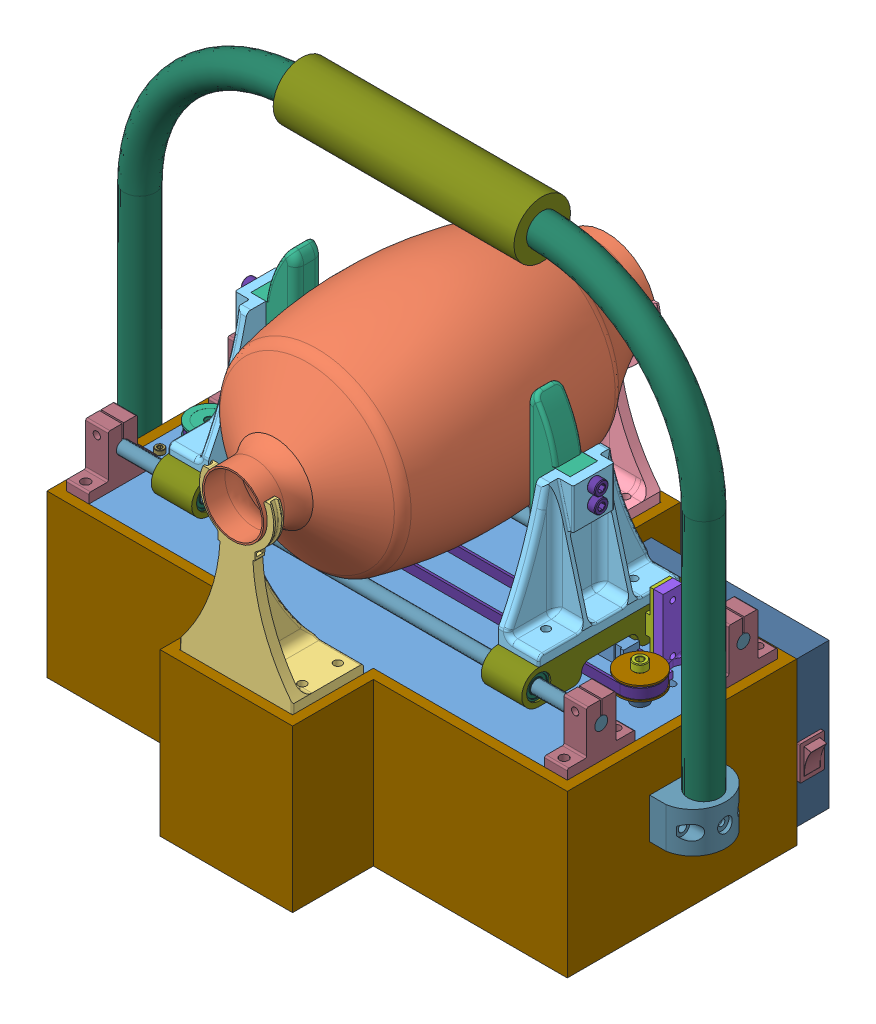
SolidWorks assembly Ensamblaje, configuration Predeterminado. Lengths in mm.
Overall size (376 340.06 240).
61 component instances, 35 part files, 118 mates.
Components (placement in the parent):
- Base-1: Base [Predeterminado] at (-72.457 -10.0807 0) size (310 6 228)
- NEMA17_2PhaseSingle-1: NEMA17_2PhaseSingle [Predeterminado] at (-200.2413 -28.7333 -47.005) size (42.3 66 52.3)
  - NEMA17-1: NEMA17 [Predeterminado] at (-3.3707 -25.3474 47) size (42.3 47 42.3)
  - Shaft-1: Shaft [Predeterminado] at (-3.3707 15.6526 47) x (-0.103422 0 0.994638) z (0 1 0) size (4.52 4.52 25)
  - cables_cover-1: cables_cover [Predeterminado] at (-3.3707 -20.3474 63.15) size (6 6 8)
  - cables-1: cables [Predeterminado] at (-3.3707 -20.3474 63.15) size (5 5 15)
- gt2 32 dientes-1: gt2 32 dientes [Конфигурация1] at (-203.612 -5.0807 -0.005) x (0 1 0) z (-0.292567 0 0.956245) size (18.5 25 25)
- Bolt M5 25mm-1: Bolt M5 25mm [M5] at (62.543 -11.5807 0) x (0.073592 0 -0.997288) z (0 1 0) size (8.5 8.5 30.5)
- 608-1: 608 [Predeterminado] at (62.543 8.9193 0) x (0.999396 0 -0.034759) z (0 -1 0) size (22 22 7)
- Tapa rod 1-1: Tapa rod 1 [Predeterminado] at (62.543 4.4193 0) x (0.973583 0 0.228334) z (-0.228334 0 0.973583) size (26 4.5 26)
- Tapa rod 1-2: Tapa rod 1 [Predeterminado] at (62.543 13.4193 0) x (0.047827 0 0.998856) z (0.998856 0 -0.047827) size (26 4.5 26)
- buje rod-1: buje rod [Predeterminado] at (62.543 4.4193 0) x (0.737781 0 -0.67504) z (0 -1 0) size (10 10 8.5)
- Nut M5-1: Nut M5 [M5] at (62.543 -12.0807 0) x (1 0 0) z (0 1 0) size (8.5 9.81 4.65)
- Bolt M3 10mm-1: Bolt M3 10mm [M3] at (-188.122 -14.0807 15.495) x (0.999941 0 -0.010855) z (0 1 0) size (5.5 5.5 13.21)
- Bolt M3 10mm-2: Bolt M3 10mm [M3] at (-219.112 -14.0807 15.495) x (0.999941 0 -0.010855) z (0 1 0) size (5.5 5.5 13.21)
- Bolt M3 10mm-3: Bolt M3 10mm [M3] at (-219.112 -14.0807 -15.495) x (0.999941 0 -0.010855) z (0 1 0) size (5.5 5.5 13.21)
- Bolt M3 10mm-4: Bolt M3 10mm [M3] at (-188.122 -14.0807 -15.495) x (0.999941 0 -0.010855) z (0 1 0) size (5.5 5.5 13.21)
- SFH8 SOPORTE-1: SFH8 SOPORTE [Default] at (-227.457 -4.0807 -44) x (0 0 -1) z (1 0 0) size (42 32.8 14)
- SFH8 SOPORTE-2: SFH8 SOPORTE [Default] at (68.543 -4.0807 -44) x (0 0 -1) z (1 0 0) size (42 32.8 14)
- SFH8 SOPORTE-3: SFH8 SOPORTE [Default] at (68.543 -4.0807 44) x (0 0 -1) z (1 0 0) size (42 32.8 14)
- SFH8 SOPORTE-4: SFH8 SOPORTE [Default] at (-227.457 -4.0807 44) x (0 0 -1) z (1 0 0) size (42 32.8 14)
- Varilla lisa-1: Varilla lisa [Predeterminado] at (82.543 15.9193 44) x (0 0 1) z (-1 0 0) size (8 8 310)
- Varilla lisa-2: Varilla lisa [Predeterminado] at (82.543 15.9193 -44) x (0 0 1) z (-1 0 0) size (8 8 310)
- LM8UU-1: LM8UU [Default] at (-185.3791 15.9193 44) x (0 -0.931414 0.363962) z (-1 0 0) size (15 15 24)
- LM8UU-2: LM8UU [Default] at (18.8571 15.9193 44) x (0 0 1) z (-1 0 0) size (15 15 24)
- LM8UU-3: LM8UU [Default] at (-185.3791 15.9193 -44) x (0 -0.940444 -0.339948) z (-1 0 0) size (15 15 24)
- LM8UU-4: LM8UU [Default] at (18.8571 15.9193 -44) x (0 0 1) z (-1 0 0) size (15 15 24)
- Guia-1: Guia [Predeterminado] at (-185.3791 15.9193 44) x (0 0 -1) z (0 -1 0) size (109 25 21)
- Guia-2: Guia [Predeterminado] at (43.8571 15.9193 -44) x (0 0 1) z (0 -1 0) size (109 25 21)
- Correa gt2-1: Correa gt2 [Predeterminado] at (-202.627 5.4193 0) x (1 0 0) z (0 1 0) size (290.17 25 6)
- Bolt M5 20mm-1: Bolt M5 20mm [M5] at (-179.3791 1.4193 8.5) x (0.741486 0 0.670968) z (0 1 0) size (8.5 8.5 25.47)
- Bolt M5 20mm-2: Bolt M5 20mm [M5] at (-166.3791 1.4193 8.5) x (1 0 0) z (0 1 0) size (8.5 8.5 25.47)
- Nut M5-2: Nut M5 [M5] at (-166.3791 3.4193 8.5) x (1 0 0) z (0 -1 0) size (8.5 9.81 4.65)
- Nut M5-3: Nut M5 [M5] at (-179.3791 3.4193 8.5) x (1 0 0) z (0 -1 0) size (8.5 9.81 4.65)
- Agarre correa-1: Agarre correa [Predeterminado] at (12.8571 10.4193 -7.5) x (0 0 -1) z (1 0 0) size (10 10 37)
- Bolt M5 20mm-3: Bolt M5 20mm [M5] at (24.8571 1.4193 -8.5) x (-0.312849 0 -0.949803) z (0 1 0) size (8.5 8.5 25.47)
- Bolt M5 20mm-4: Bolt M5 20mm [M5] at (37.8571 1.4193 -8.5) x (0.801692 0 0.597737) z (0 1 0) size (8.5 8.5 25.47)
- Ambu-1: Ambu [Predeterminado] at (-106.269 45.8029 -63.7938) x (0.596879 0.802331 0) z (0.802331 -0.596879 0) size (130.8 231 130.8)
- Soporte 1-1: Soporte 1 [Predeterminado] at (-72.4573 -4.2227 90) x (0.999992 -0.004057 0) z (0 0 1) size (71.01 106.02 44.55)
- Soporte 2-1: Soporte 2 [Predeterminado] at (-72.457 -4.0807 -88) x (-1 0 0) z (0 0 -1) size (73.4 106.02 44.28)
- Soporte brazo-1: Soporte brazo [Predeterminado] at (31.3571 26.4193 0) x (0 0 -1) z (1 0 0) size (88 76.5 25.25)
- Soporte brazo-2: Soporte brazo [Predeterminado] at (-172.8791 26.4193 0) x (0 0 1) z (-1 0 0) size (88 76.5 25.25)
- Garra-1: Garra [Predeterminado] at (-89.5176 97.1445 -8.45) x (1 0 0) z (0 -1 0) size (27.74 17.58 79.53)
- Garra-2: Garra [Predeterminado] at (-52.3557 97.1445 8.55) x (-1 0 0) z (0 -1 0) size (27.74 17.58 79.53)
- Fin de carrera-1: Fin de carrera [Predeterminado] at (48.7353 16.9193 -28.1) x (0 1 0) z (0 0 1) size (42 18.5 12)
- Soporte Fin de carrera-1: Soporte Fin de carrera [Predeterminado] at (48.7353 16.9193 -28.1) x (0 0 -1) z (1 0 0) size (24 42 12)
- Caja-1: Caja [Predeterminado] at (-72.457 -104.0807 1) x (1 0 0) z (0 1 0) size (322 240 100)
- Gabinete-1: Gabinete [Predeterminado] at (28.543 -54.0807 -96) x (1 0 0) z (0 -1 0) size (110 25 90)
- LCDmodule-1: LCDmodule [Default] at (-11.457 -33.6807 -87.35) x (1 0 0) z (0 1 0) size (82.75 18.75 36)
- potenciometro-1: potenciometro [Predeterminado] at (28.543 -72.0807 -82.5) x (-1 0 0) z (0 0 -1) size (17 25.3 29.7)
- potenciometro-2: potenciometro [Predeterminado] at (58.543 -72.0807 -82.5) x (-1 0 0) z (0 0 -1) size (17 25.3 29.7)
- potenciometro-3: potenciometro [Predeterminado] at (-1.457 -72.0807 -82.5) x (-1 0 0) z (0 0 -1) size (17 25.3 29.7)
- Interruptor-1: Interruptor [Predeterminado] at (83.543 -64.5807 -83.75) x (0 -1 0) z (0 0 1) size (21 17.27 15)
- Soporte barra-1: Soporte barra [Predeterminado] at (102.043 -56.5807 0) x (0 0 -1) z (0 1 0) size (40 27 25)
- Soporte barra-2: Soporte barra [Predeterminado] at (-246.957 -56.5807 0) x (0 0 1) z (0 1 0) size (40 27 25)
- Barra-1: Barra [Predeterminado] at (-246.957 -31.5238 0) size (368.5 259.75 19.5)
- manopla-1: manopla [Predeterminado] at (-146.957 218.4762 0) x (0 0 -1) z (1 0 0) size (35 35 149)
- Bolt M5 30mm-1: Bolt M5 30mm [M5] at (-145.3791 97.9193 0) x (0 0.924225 0.381849) z (-1 0 0) size (8.5 8.5 35.53)
- Bolt M5 30mm-2: Bolt M5 30mm [M5] at (-145.3791 88.1193 0) x (0 0.924225 0.381849) z (-1 0 0) size (8.5 8.5 35.53)
- Bolt M5 30mm-3: Bolt M5 30mm [M5] at (3.857 97.9193 0) x (0 -0.924225 -0.381849) z (1 0 0) size (8.5 8.5 35.53)
- Bolt M5 30mm-4: Bolt M5 30mm [M5] at (3.857 88.1193 0) x (0 -0.924225 -0.381849) z (1 0 0) size (8.5 8.5 35.53)
Mates (geometry in assembly coordinates):
- Coincidente1: coincident: plane of assembly; plane of assembly; plane of Base-1 through (-72.457 -10.0807 0) normal (0 -1 0); plane of NEMA17_2PhaseSingle-1/NEMA17-1 through (-203.612 -10.0807 -0.005) normal (0 1 0)
- Concéntrica4: concentric: circle of assembly; circle of assembly; circle of Base-1; circle of NEMA17_2PhaseSingle-1/NEMA17-1
- Concéntrica7: concentric: circle of assembly; circle of assembly; circle of Base-1; circle of NEMA17_2PhaseSingle-1/NEMA17-1
- Concéntrica8: concentric: cylinder of assembly; cylinder of assembly; cylinder of NEMA17_2PhaseSingle-1/Shaft-1 through (-203.612 11.9193 -0.005) axis (0 -1 0) radius 2.26; cylinder of gt2 32 dientes-1 through (-203.612 -5.0807 -0.005) axis (0 1 0) radius 2.65
- Distancia1: distance = 2 mm: plane of assembly; plane of assembly; plane of NEMA17_2PhaseSingle-1/NEMA17-1 through (-203.612 -7.0807 -0.005) normal (0 1 0); plane of gt2 32 dientes-1 through (-203.612 -5.0807 -0.005) normal (0 -1 0)
- Concéntrica9: concentric: cylinder of assembly; circle of assembly; cylinder of Base-1 through (62.543 -4.0807 0) axis (0 -1 0) radius 2.65; circle of Bolt M5 25mm-1
- Concéntrica10: concentric: cylinder of assembly; cylinder of assembly; cylinder of Bolt M5 25mm-1 through (62.543 18.4193 0) axis (0 -1 0) radius 4.25; cylinder of 608-1 through (62.543 5.4193 0) axis (0 1 0) radius 4
- Distancia2: distance = 9.5 mm: plane of assembly; plane of assembly; plane of 608-1 through (62.543 5.4193 0) normal (0 -1 0); plane of Base-1 through (-72.457 -4.0807 0) normal (0 1 0)
- Concéntrica11: concentric: circle of assembly; circle of assembly; circle of 608-1; circle of Tapa rod 1-1
- Coincidente4: coincident: plane of assembly; plane of assembly; plane of 608-1 through (62.543 5.4193 0) normal (0 -1 0); plane of Tapa rod 1-1 through (62.543 5.4193 0) normal (0 1 0)
- Coincidente5: coincident: plane of assembly; plane of assembly; plane of 608-1 through (62.543 12.4193 0) normal (0 1 0); plane of Tapa rod 1-2 through (62.543 12.4193 0) normal (0 -1 0)
- Concéntrica12: concentric: circle of assembly; circle of assembly; circle of 608-1; circle of Tapa rod 1-2
- Concéntrica13: concentric: cylinder of assembly; cylinder of assembly; cylinder of Bolt M5 25mm-1 through (62.543 18.4193 0) axis (0 -1 0) radius 4.25; cylinder of buje rod-1 through (62.543 -4.0807 0) axis (0 1 0) radius 2.65
- Coincidente6: coincident: plane of assembly; plane of assembly; plane of Base-1 through (-72.457 -4.0807 0) normal (0 1 0); plane of buje rod-1 through (62.543 -4.0807 0) normal (0 -1 0)
- Coincidente7: coincident: plane of assembly; plane of assembly; plane of Bolt M5 25mm-1 through (62.543 13.4193 0) normal (0 -1 0); plane of Tapa rod 1-2 through (62.543 13.4193 0) normal (0 1 0)
- Coincidente8: coincident: plane of assembly; plane of assembly; plane of Base-1 through (-72.457 -10.0807 0) normal (0 -1 0); plane of Nut M5-1 through (62.543 -10.0807 0) normal (0 1 0)
- Concéntrica14: concentric: circle of assembly; circle of assembly; circle of Bolt M5 25mm-1; circle of Nut M5-1
- Concéntrica15: concentric: circle of assembly; circle of assembly; circle of Base-1; circle of Bolt M3 10mm-1
- Coincidente9: coincident: plane of assembly; plane of assembly; plane of Base-1 through (-72.457 -4.0807 0) normal (0 1 0); plane of Bolt M3 10mm-1 through (-188.122 -4.0807 15.495) normal (0 -1 0)
- Coincidente10: coincident: line of assembly; line of assembly; line of Base-1 through (-107.457 -4.0807 -65) axis (-1 0 0); line of SFH8 SOPORTE-1 through (-213.457 -4.0807 -65) axis (-1 0 0)
- Coincidente11: coincident: plane of assembly; plane of assembly; plane of Base-1 through (-72.457 -4.0807 0) normal (0 1 0); plane of SFH8 SOPORTE-1 through (-213.457 -4.0807 -23) normal (0 -1 0)
- Coincidente12: coincident: line of assembly; line of assembly; line of Base-1 through (-227.457 -4.0807 -65) axis (0 0 1); line of SFH8 SOPORTE-1 through (-227.457 -4.0807 -23) axis (0 0 -1)
- Concéntrica16: concentric: cylinder of assembly; cylinder of assembly; cylinder of SFH8 SOPORTE-4 through (-213.457 15.9193 44) axis (-1 0 0) radius 4; cylinder of Varilla lisa-1 through (-227.457 15.9193 44) axis (1 0 0) radius 4
- Coincidente13: coincident: plane of assembly; plane of assembly; plane of SFH8 SOPORTE-3 through (82.543 15.9193 44) normal (1 0 0); plane of Varilla lisa-1 through (82.543 15.9193 44) normal (1 0 0)
- Concéntrica17: concentric: cylinder of assembly; cylinder of assembly; cylinder of SFH8 SOPORTE-2 through (82.543 15.9193 -44) axis (-1 0 0) radius 4; cylinder of Varilla lisa-2 through (-227.457 15.9193 -44) axis (1 0 0) radius 4
- Coincidente14: coincident: plane of assembly; plane of assembly; plane of SFH8 SOPORTE-2 through (82.543 15.9193 -44) normal (1 0 0); plane of Varilla lisa-2 through (82.543 15.9193 -44) normal (1 0 0)
- Concéntrica18: concentric: cylinder of assembly; cylinder of assembly; cylinder of Varilla lisa-1 through (-227.457 15.9193 44) axis (1 0 0) radius 4; cylinder of LM8UU-1 through (-161.3791 15.9193 44) axis (-1 0 0) radius 4
- Concéntrica19: concentric: cylinder of assembly; cylinder of assembly; cylinder of Varilla lisa-1 through (-227.457 15.9193 44) axis (1 0 0) radius 4; cylinder of LM8UU-2 through (42.8571 15.9193 44) axis (-1 0 0) radius 4
- Concéntrica20: concentric: cylinder of assembly; cylinder of assembly; cylinder of Varilla lisa-2 through (-227.457 15.9193 -44) axis (1 0 0) radius 4; cylinder of LM8UU-3 through (-161.3791 15.9193 -44) axis (-1 0 0) radius 4
- Concéntrica21: concentric: cylinder of assembly; cylinder of assembly; cylinder of Varilla lisa-2 through (-227.457 15.9193 -44) axis (1 0 0) radius 4; cylinder of LM8UU-4 through (42.8571 15.9193 -44) axis (-1 0 0) radius 4
- Concéntrica22: concentric: cylinder of assembly; cylinder of assembly; cylinder of LM8UU-3 through (-161.3791 15.9193 -44) axis (-1 0 0) radius 7.5; cylinder of Guia-1 through (-160.3791 15.9193 -44) axis (-1 0 0) radius 7.5
- Concéntrica23: concentric: cylinder of assembly; cylinder of assembly; cylinder of LM8UU-1 through (-161.3791 15.9193 44) axis (-1 0 0) radius 7.5; cylinder of Guia-1 through (-160.3791 15.9193 44) axis (-1 0 0) radius 7.5
- Concéntrica26: concentric: cylinder of assembly; cylinder of assembly; cylinder of 608-1 through (62.543 5.4193 0) axis (0 1 0) radius 11; cylinder of Correa gt2-1 through (62.543 11.4193 0) axis (0 -1 0) radius 11
- Coincidente19: coincident: plane of assembly; plane of assembly; plane of Tapa rod 1-1 through (62.543 5.4193 0) normal (0 1 0); plane of Correa gt2-1 through (62.543 5.4193 0) normal (0 -1 0)
- Paralelo1: parallel: plane of assembly; plane of assembly; plane of SFH8 SOPORTE-4 through (-213.457 28.7193 35) normal (0 0 -1); plane of Correa gt2-1 through (-202.627 11.4193 12.5) normal (0 0 1)
- Coincidente29: coincident: plane of assembly; plane of assembly; plane of LM8UU-3 through (-185.3791 15.9193 -44) normal (-1 0 0); plane of Guia-1 through (-185.3791 15.9193 -44) normal (-1 0 0)
- Coincidente31: coincident: plane of assembly; plane of assembly; plane of LM8UU-1 through (-185.3791 15.9193 44) normal (-1 0 0); plane of Guia-1 through (-185.3791 15.9193 -44) normal (-1 0 0)
- Concéntrica32: concentric: cylinder of assembly; cylinder of assembly; cylinder of Guia-1 through (-179.3791 21.4193 8.5) axis (0 1 0) radius 4.375; cylinder of Bolt M5 20mm-1 through (-179.3791 26.4193 8.5) axis (0 -1 0) radius 4.25
- Coincidente34: coincident: plane of assembly; plane of assembly; plane of Guia-1 through (-179.3791 21.4193 8.5) normal (0 1 0); plane of Bolt M5 20mm-1 through (-179.3791 21.4193 8.5) normal (0 -1 0)
- Concéntrica33: concentric: cylinder of assembly; cylinder of assembly; cylinder of Guia-1 through (-166.3791 21.4193 8.5) axis (0 1 0) radius 4.375; cylinder of Bolt M5 20mm-2 through (-166.3791 26.4193 8.5) axis (0 -1 0) radius 4.25
- Coincidente35: coincident: plane of assembly; plane of assembly; plane of Bolt M5 20mm-1 through (-179.3791 26.4193 8.5) normal (0 1 0); plane of Bolt M5 20mm-2 through (-166.3791 26.4193 8.5) normal (0 1 0)
- Concéntrica34: concentric: cylinder of assembly; cylinder of assembly; cylinder of LM8UU-4 through (42.8571 15.9193 -44) axis (-1 0 0) radius 7.5; cylinder of Guia-2 through (18.8571 15.9193 -44) axis (1 0 0) radius 7.5
- Coincidente36: coincident: plane of assembly; plane of assembly; plane of LM8UU-4 through (18.8571 15.9193 -44) normal (-1 0 0); plane of Guia-2 through (18.8571 15.9193 44) normal (-1 0 0)
- Concéntrica35: concentric: cylinder of assembly; cylinder of assembly; cylinder of LM8UU-2 through (42.8571 15.9193 44) axis (-1 0 0) radius 7.5; cylinder of Guia-2 through (18.8571 15.9193 44) axis (1 0 0) radius 7.5
- Coincidente37: coincident: plane of assembly; plane of assembly; plane of LM8UU-2 through (18.8571 15.9193 44) normal (-1 0 0); plane of Guia-2 through (18.8571 15.9193 44) normal (-1 0 0)
- Concéntrica36: concentric: circle of assembly; circle of assembly; circle of Bolt M5 20mm-2; circle of Nut M5-2
- Coincidente38: coincident: plane of assembly; plane of assembly; plane of Bolt M5 20mm-2 through (-166.3791 1.4193 8.5) normal (0 -1 0); plane of Nut M5-2 through (-166.3791 1.4193 8.5) normal (0 -1 0)
- Concéntrica38: concentric: circle of assembly; circle of assembly; circle of Bolt M5 20mm-1; circle of Nut M5-3
- Coincidente39: coincident: plane of assembly; plane of assembly; plane of Bolt M5 20mm-1 through (-179.3791 1.4193 8.5) normal (0 -1 0); plane of Nut M5-3 through (-179.3791 1.4193 8.5) normal (0 -1 0)
- Coincidente40: coincident: cylinder of assembly; circle of assembly; cylinder of Guia-2 through (24.8571 5.4193 -8.5) axis (0 1 0) radius 2.5; circle of Agarre correa-1
- Coincidente41: coincident: plane of assembly; plane of assembly; plane of Guia-2 through (18.8571 15.4193 -17.5) normal (0 -1 0); plane of Agarre correa-1 through (49.8571 15.4193 -2.5) normal (0 1 0)
- Concéntrica39: concentric: cylinder of assembly; cylinder of assembly; cylinder of Guia-2 through (37.8571 5.4193 -8.5) axis (0 1 0) radius 2.5; cylinder of Agarre correa-1 through (37.8571 5.4193 -8.5) axis (0 1 0) radius 2.5
- Concéntrica41: concentric: cylinder of assembly; cylinder of assembly; cylinder of Guia-2 through (24.8571 21.4193 -8.5) axis (0 1 0) radius 4.375; cylinder of Bolt M5 20mm-3 through (24.8571 26.4193 -8.5) axis (0 -1 0) radius 4.25
- Coincidente44: coincident: plane of assembly; plane of assembly; plane of Guia-2 through (18.8571 26.4193 44) normal (0 1 0); plane of Bolt M5 20mm-3 through (24.8571 26.4193 -8.5) normal (0 1 0)
- Concéntrica42: concentric: cylinder of assembly; cylinder of assembly; cylinder of Guia-2 through (37.8571 21.4193 -8.5) axis (0 1 0) radius 4.375; cylinder of Bolt M5 20mm-4 through (37.8571 26.4193 -8.5) axis (0 -1 0) radius 4.25
- Coincidente45: coincident: plane of assembly; plane of assembly; plane of Guia-2 through (18.8571 26.4193 44) normal (0 1 0); plane of Bolt M5 20mm-4 through (37.8571 26.4193 -8.5) normal (0 1 0)
- Coincidente49: coincident: line of assembly; line of assembly; line of Base-1 through (-107.457 -4.0807 65) axis (0 0 1); line of Soporte 1-1 through (-107.457 -4.0807 71) axis (0 0 1)
- Coincidente50: coincident: plane of assembly; plane of assembly; plane of Base-1 through (-43.457 -4.0807 115) normal (0 0 1); plane of Soporte 1-1 through (51.0357 72.2482 115) normal (0 0 1)
- Concéntrica44: concentric: cylinder of assembly; cylinder of assembly; cylinder of Ambu-1 through (-72.0678 91.7765 -63.7938) axis (0 0 -1) radius 19; cylinder of Soporte 1-1 through (-72.0678 91.7765 115) axis (0 0 -1) radius 19
- Coincidente52: coincident: line of assembly; line of assembly; line of Base-1 through (-107.457 -4.0807 -113) axis (0 0 1); line of Soporte 2-1 through (-107.457 -4.0807 -112) axis (0 0 1)
- Coincidente53: coincident: plane of assembly; plane of assembly; plane of Base-1 through (-72.457 -4.0807 0) normal (0 1 0); plane of Soporte 2-1 through (-72.457 -4.0807 -88) normal (0 -1 0)
- Coincidente54: coincident: line of assembly; line of assembly; line of Base-1 through (-37.457 -4.0807 -113) axis (-1 0 0); line of Soporte 2-1 through (-38.457 -4.0807 -113) axis (-1 0 0)
- Coincidente55: coincident: plane of assembly; plane of assembly; plane of Guia-2 through (18.8571 15.9193 44) normal (-1 0 0); plane of Soporte brazo-1 through (18.8571 32.4193 44) normal (-1 0 0)
- Coincidente56: coincident: plane of assembly; plane of assembly; plane of Guia-2 through (18.8571 26.4193 44) normal (0 1 0); plane of Soporte brazo-1 through (31.3571 26.4193 0) normal (0 -1 0)
- Concéntrica45: concentric: cylinder of assembly; cylinder of assembly; cylinder of Guia-2 through (31.3571 5.4193 -27) axis (0 1 0) radius 2.6; cylinder of Soporte brazo-1 through (31.3571 102.9193 -27) axis (0 -1 0) radius 2.5
- Coincidente57: coincident: plane of assembly; plane of assembly; plane of Guia-1 through (-160.3791 15.9193 -44) normal (1 0 0); plane of Soporte brazo-2 through (-160.3791 32.4193 -44) normal (1 0 0)
- Coincidente58: coincident: plane of assembly; plane of assembly; plane of Guia-1 through (-160.3791 26.4193 -44) normal (0 1 0); plane of Soporte brazo-2 through (-172.8791 26.4193 0) normal (0 -1 0)
- Concéntrica46: concentric: cylinder of assembly; cylinder of assembly; cylinder of Guia-1 through (-172.8791 5.4193 -27) axis (0 1 0) radius 2.6; cylinder of Soporte brazo-2 through (-172.8791 102.9193 -27) axis (0 -1 0) radius 2.5
- Coincidente60: coincident: plane of assembly; plane of assembly; plane of Soporte brazo-2 through (-157.3791 82.9193 8.55) normal (0 0 -1); plane of Garra-1 through (-87.4092 92.9193 8.55) normal (0 0 1)
- Coincidente64: coincident: plane of assembly; plane of assembly; plane of Soporte brazo-1 through (15.8571 82.9193 8.55) normal (0 0 -1); plane of Garra-2 through (-54.4641 92.9193 8.55) normal (0 0 1)
- Coincidente68: coincident: plane of assembly; plane of assembly; plane of Soporte brazo-2 through (-172.8791 102.9193 0) normal (0 1 0); plane of Garra-1 through (-160.7304 102.9193 8.55) normal (0 1 0)
- Paralelo2: parallel: plane of assembly; plane of assembly; plane of Guia-2 through (43.8571 15.9193 44) normal (1 0 0); plane of Fin de carrera-1 through (39.7353 16.9193 -28.1) normal (-1 0 0)
- Paralelo3: parallel: plane of assembly; plane of assembly; plane of Base-1 through (-21.457 -4.0807 -65) normal (0 0 -1); plane of Fin de carrera-1 through (46.7353 -4.0807 -34.1) normal (0 0 -1)
- Paralelo4: parallel: plane of assembly; plane of assembly; plane of Fin de carrera-1 through (48.7353 16.9193 -28.1) normal (1 0 0); plane of Soporte Fin de carrera-1 through (48.7353 16.9193 -28.1) normal (-1 0 0)
- Coincidente73: coincident: plane of assembly; plane of assembly; plane of Base-1 through (-72.457 -4.0807 0) normal (0 1 0); plane of Soporte Fin de carrera-1 through (54.7353 -4.0807 -22.1) normal (0 -1 0)
- Concéntrica48: concentric: cylinder of assembly; cylinder of assembly; cylinder of Fin de carrera-1 through (46.7353 31.9193 -28.1) axis (1 0 0) radius 1.6; cylinder of Soporte Fin de carrera-1 through (48.7353 31.9193 -28.1) axis (1 0 0) radius 1.75
- Coincidente74: coincident: plane of assembly; plane of assembly; plane of Fin de carrera-1 through (48.7353 16.9193 -28.1) normal (1 0 0); plane of Soporte Fin de carrera-1 through (48.7353 16.9193 -28.1) normal (-1 0 0)
- Tangente2: tangent: plane of assembly; cylinder of assembly; plane of Base-1 through (63.543 -10.0807 -17) normal (0 0 -1); cylinder of Soporte Fin de carrera-1 through (57.7353 -0.0807 -19.1) axis (0 -1 0) radius 2.1
- Paralelo5: parallel: plane of assembly; plane of assembly; plane of Base-1 through (-72.457 -10.0807 0) normal (0 -1 0); plane of Caja-1 through (-72.457 -98.0807 1) normal (0 1 0)
- Paralelo6: parallel: plane of assembly; plane of assembly; plane of Base-1 through (-21.457 -4.0807 -65) normal (0 0 -1); plane of Caja-1 through (88.543 -4.0807 -71) normal (0 0 -1)
- Coincidente78: coincident: point of assembly; point of assembly; point of Base-1; point of Caja-1
- Coincidente81: coincident: plane of assembly; plane of assembly; plane of Gabinete-1 through (65.993 -18.2307 -89) normal (0 0 1); plane of LCDmodule-1 through (-11.457 -33.6807 -89) normal (0 0 -1)
- Concéntrica51: concentric: cylinder of assembly; cylinder of assembly; cylinder of Gabinete-1 through (65.993 -18.2307 -96) axis (0 0 1) radius 0.95; cylinder of LCDmodule-1 through (65.993 -18.2307 -84) axis (0 0 -1) radius 1.45
- Concéntrica52: concentric: cylinder of assembly; cylinder of assembly; cylinder of Gabinete-1 through (65.993 -49.1307 -96) axis (0 0 1) radius 0.95; cylinder of LCDmodule-1 through (65.993 -49.1307 -84) axis (0 0 -1) radius 1.45
- Concéntrica53: concentric: cylinder of assembly; cylinder of assembly; cylinder of Gabinete-1 through (28.543 -72.0807 -71) axis (0 0 -1) radius 3.6; cylinder of potenciometro-1 through (28.543 -72.0807 -99) axis (0 0 -1) radius 2.5
- Paralelo8: parallel: plane of assembly; plane of assembly; plane of Gabinete-1 through (80.543 -99.0807 -71) normal (-1 0 0); plane of potenciometro-1 through (33.043 -84.5807 -83.9) normal (-1 0 0)
- Coincidente83: coincident: plane of assembly; plane of assembly; plane of Gabinete-1 through (28.543 -54.0807 -93) normal (0 0 1); plane of potenciometro-1 through (28.543 -72.0807 -93) normal (0 0 -1)
- Concéntrica54: concentric: cylinder of assembly; cylinder of assembly; cylinder of Gabinete-1 through (58.543 -72.0807 -71) axis (0 0 -1) radius 3.6; cylinder of potenciometro-2 through (58.543 -72.0807 -93) axis (0 0 1) radius 5
- Coincidente84: coincident: plane of assembly; plane of assembly; plane of Gabinete-1 through (28.543 -54.0807 -93) normal (0 0 1); plane of potenciometro-2 through (58.543 -72.0807 -93) normal (0 0 -1)
- Concéntrica55: concentric: cylinder of assembly; cylinder of assembly; cylinder of Gabinete-1 through (-1.457 -72.0807 -71) axis (0 0 -1) radius 3.6; cylinder of potenciometro-3 through (-1.457 -72.0807 -93) axis (0 0 1) radius 5
- Coincidente85: coincident: plane of assembly; plane of assembly; plane of Gabinete-1 through (28.543 -54.0807 -93) normal (0 0 1); plane of potenciometro-3 through (-1.457 -72.0807 -93) normal (0 0 -1)
- Paralelo9: parallel: plane of assembly; plane of assembly; plane of Caja-1 through (-72.457 -4.0807 1) normal (0 1 0); plane of Gabinete-1 through (-26.457 -9.0807 -71) normal (0 1 0)
- Coincidente87: coincident: plane of assembly; plane of assembly; plane of Caja-1 through (88.543 -4.0807 -71) normal (0 0 -1); plane of Gabinete-1 through (28.543 -54.0807 -71) normal (0 0 1)
- Coincidente89: coincident: plane of assembly; plane of assembly; plane of Gabinete-1 through (73.543 -74.0807 -89.75) normal (0 0 1); plane of Interruptor-1 through (73.043 -56.0807 -89.75) normal (0 0 -1)
- Coincidente90: coincident: plane of assembly; plane of assembly; plane of Gabinete-1 through (83.543 -99.0807 -71) normal (1 0 0); plane of Interruptor-1 through (83.543 -54.5807 -76.75) normal (-1 0 0)
- Paralelo10: parallel: plane of assembly; plane of assembly; plane of potenciometro-1 through (36.043 -83.5807 -83.5) normal (1 0 0); plane of potenciometro-2 through (51.043 -83.5807 -83.5) normal (-1 0 0)
- Paralelo11: parallel: plane of assembly; plane of assembly; plane of potenciometro-1 through (21.043 -83.5807 -83.5) normal (-1 0 0); plane of potenciometro-3 through (6.043 -83.5807 -83.5) normal (1 0 0)
- Coincidente93: coincident: line of assembly; line of assembly; line of Gabinete-1 through (83.543 -54.0807 -89.75) axis (0 0 1); line of Interruptor-1 through (83.543 -54.0807 -90.75) axis (0 0 1)
- Concéntrica56: concentric: cylinder of assembly; cylinder of assembly; cylinder of Caja-1 through (78.543 -14.0807 -65) axis (0 0 -1) radius 1.5; cylinder of Gabinete-1 through (78.543 -14.0807 -96) axis (0 0 1) radius 1.6
- Coincidente94: coincident: plane of assembly; plane of assembly; plane of Caja-1 through (88.543 -4.0807 71) normal (1 0 0); plane of Soporte barra-1 through (88.543 -31.5807 0) normal (-1 0 0)
- Concéntrica57: concentric: cylinder of assembly; cylinder of assembly; cylinder of Caja-1 through (-233.457 -44.0807 -14.75) axis (1 0 0) radius 2.6; cylinder of Soporte barra-1 through (88.543 -44.0807 -14.75) axis (1 0 0) radius 2.6
- Concéntrica58: concentric: cylinder of assembly; cylinder of assembly; cylinder of Caja-1 through (-233.457 -44.0807 14.75) axis (1 0 0) radius 2.6; cylinder of Soporte barra-1 through (88.543 -44.0807 14.75) axis (1 0 0) radius 2.6
- Coincidente95: coincident: plane of assembly; plane of assembly; plane of Caja-1 through (-233.457 -4.0807 -71) normal (-1 0 0); plane of Soporte barra-2 through (-233.457 -31.5807 0) normal (1 0 0)
- Concéntrica59: concentric: cylinder of assembly; cylinder of assembly; cylinder of Caja-1 through (-233.457 -44.0807 14.75) axis (1 0 0) radius 2.6; cylinder of Soporte barra-2 through (-233.457 -44.0807 14.75) axis (-1 0 0) radius 2.6
- Concéntrica60: concentric: cylinder of assembly; cylinder of assembly; cylinder of Caja-1 through (-233.457 -44.0807 -14.75) axis (1 0 0) radius 2.6; cylinder of Soporte barra-2 through (-233.457 -44.0807 -14.75) axis (-1 0 0) radius 2.6
- Concéntrica61: concentric: circle of assembly; circle of assembly; circle of Soporte barra-2; circle of Barra-1
- Concéntrica62: concentric: circle of assembly; circle of assembly; circle of Soporte barra-1; circle of Barra-1
- Concéntrica63: concentric: cylinder of assembly; cylinder of assembly; cylinder of Barra-1 through (-146.957 218.4762 0) axis (1 0 0) radius 9.75; cylinder of manopla-1 through (2.043 218.4762 0) axis (-1 0 0) radius 9.75
- Coincidente96: coincident: circle of assembly; circle of assembly; circle of Barra-1; circle of manopla-1
- Coincidente97: coincident: plane of assembly; plane of assembly; plane of Soporte brazo-1 through (27.8571 26.4193 0) normal (-1 0 0); plane of Garra-2 through (27.8571 82.9193 -8.45) normal (1 0 0)
- Concéntrica64: concentric: cylinder of assembly; cylinder of assembly; cylinder of Soporte brazo-2 through (-185.634 97.9193 0) axis (1 0 0) radius 2.6; cylinder of Bolt M5 30mm-1 through (-180.3791 97.9193 0) axis (1 0 0) radius 4.25
- Coincidente98: coincident: plane of assembly; plane of assembly; plane of Soporte brazo-2 through (-175.3791 77.9193 -12.75) normal (-1 0 0); plane of Bolt M5 30mm-1 through (-175.3791 97.9193 0) normal (1 0 0)
- Concéntrica65: concentric: cylinder of assembly; cylinder of assembly; cylinder of Soporte brazo-2 through (-185.634 88.1193 0) axis (1 0 0) radius 2.6; cylinder of Bolt M5 30mm-2 through (-180.3791 88.1193 0) axis (1 0 0) radius 4.25
- Coincidente99: coincident: plane of assembly; plane of assembly; plane of Soporte brazo-2 through (-175.3791 77.9193 -12.75) normal (-1 0 0); plane of Bolt M5 30mm-2 through (-175.3791 88.1193 0) normal (1 0 0)
- Concéntrica66: concentric: cylinder of assembly; cylinder of assembly; cylinder of Soporte brazo-1 through (44.1119 97.9193 0) axis (-1 0 0) radius 2.6; cylinder of Bolt M5 30mm-3 through (38.857 97.9193 0) axis (-1 0 0) radius 4.25
- Coincidente100: coincident: plane of assembly; plane of assembly; plane of Soporte brazo-1 through (33.857 77.9193 12.75) normal (1 0 0); plane of Bolt M5 30mm-3 through (33.857 97.9193 0) normal (-1 0 0)
- Concéntrica67: concentric: cylinder of assembly; cylinder of assembly; cylinder of Soporte brazo-1 through (44.1119 88.1193 0) axis (-1 0 0) radius 2.6; cylinder of Bolt M5 30mm-4 through (38.857 88.1193 0) axis (-1 0 0) radius 4.25
- Coincidente101: coincident: plane of assembly; plane of assembly; plane of Soporte brazo-1 through (33.857 77.9193 12.75) normal (1 0 0); plane of Bolt M5 30mm-4 through (33.857 88.1193 0) normal (-1 0 0)
